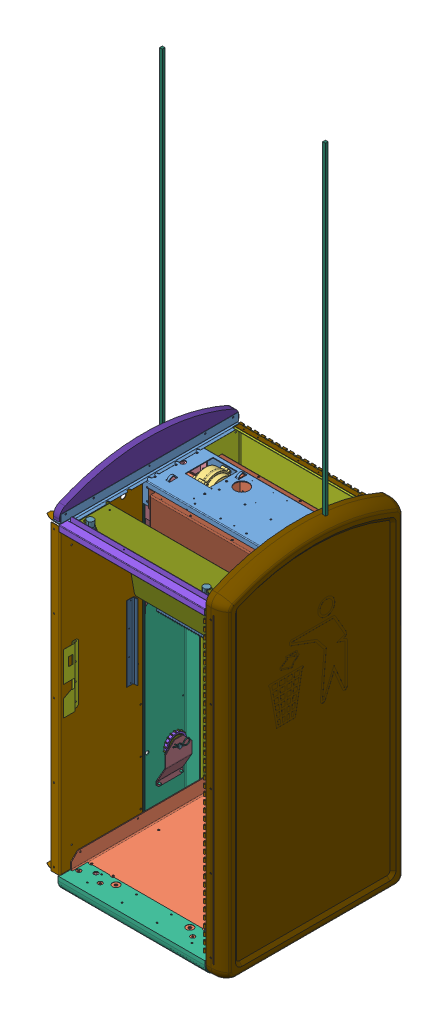
SolidWorks assembly BB3_Assy_Meca_3D, configuration Défaut. Lengths in mm.
Overall size (667 1195.8 661.5).
120 component instances, 56 part files, 9 mates.
Components (placement in the parent):
- BB3_Chassis-1: BB3_Chassis [Défaut] at (-140.0351 388.7943 -82.8142) size (675.82 1282.03 663.93)
  - TopCrossmember_Rev2-1: TopCrossmember_Rev2 [Default] at (20.5473 102.5902 0) size (635 86.99 210.82)
  - TopCrossMotorBrkt_Rev3-1: TopCrossMotorBrkt_Rev3 [Défaut] at (-101.9976 61.051 0) size (152.4 200.54 205.51)
  - Moto_Reducteur_011_562_1_216-1: Moto_Reducteur_011_562_1_216 [Default] at (192.9322 74.2423 -36.8146) x (0 -0.000019 -1) z (-1 0 0) size (114.3 226.4 239.81)
  - TopCrossBearingBrkt_Rev1-1: TopCrossBearingBrkt_Rev1 [Défaut] at (-246.0257 61.051 0) size (25.4 73.66 205.51)
  - TopCrossBearingBrkt_Rev1-2: TopCrossBearingBrkt_Rev1 [Défaut] at (287.1203 61.051 0) x (-1 0 0) z (0 0 -1) size (25.4 73.66 205.51)
  - Chassis_Coussinet-1: Chassis_Coussinet [Default] at (-247.5497 60.2788 -36.8146) x (0 -0.995993 0.089436) z (0 0.089436 0.995993) size (28.27 19.05 28.27)
  - Chassis_Coussinet-2: Chassis_Coussinet [Default] at (288.6443 60.2788 -36.8146) x (0 0.997938 0.064185) z (0 -0.064185 0.997938) size (28.27 19.05 28.27)
  - Chassis_Support_Moteur-1: Chassis_Support_Moteur [Défaut] at (-296.9017 100.6288 0.0002) x (0 0 1) z (0 1 0) size (205.51 54 1127)
  - Chassis_Support_Moteur-2: Chassis_Support_Moteur [Défaut] at (337.9963 100.6288 0.0002) x (0 0 -1) z (0 1 0) size (205.51 54 1127)
  - Chassis_Panneau_Arriere-2: Chassis_Panneau_Arriere [Défaut] at (20.5983 -479.4712 -246.619) x (0 0 1) z (0 1 0) size (164.98 667 1155.29)
  - Chassis_Support_Batterie-2: Chassis_Support_Batterie [Défaut] at (20.5983 -270.8192 -242.544) x (0 0 1) z (-1 0 0) size (116.32 446 529)
  - Chassis_Support_Moteur_Devant_Gauche-2: Chassis_Support_Moteur_Devant_Gauche [Défaut] at (-249.8894 -442.8187 130.7585) x (0 0 -1) z (0 1 0) size (329.85 66 1105)
  - Chassis_Positionnement_Emetteur_Recepteur_Gauche-2: Chassis_Positionnement_Emetteur_Recepteur_Gauche [Défaut] at (-222.4622 -381.8185 156.8606) x (1 0 0) z (0 -1 0) size (22.1 48.5 273)
  - Chassis_Support_Moteur_Devant_Droite-1: Chassis_Support_Moteur_Devant_Droite [Défaut] at (290.9839 -442.8187 130.7585) x (0 0 -1) z (0 -1 0) size (329.85 66 1105)
  - Chassis_Positionnement_Emetteur_Recepteur_Droite-1: Chassis_Positionnement_Emetteur_Recepteur_Droite [Défaut] at (263.5568 -381.8185 156.8606) x (-1 0 0) z (0 1 0) size (22.1 48.5 273)
  - Chassis_Support_Pignon_bas-1: Chassis_Support_Pignon_bas [Défaut] at (305.4963 -865.3715 -39.8528) x (-1 0 0) z (0 0 1) size (35.2 151.29 95)
  - Chassis_Axe_Pignon_Bas-1: Chassis_Axe_Pignon_Bas [Défaut] at (340.9963 -816.3715 -39.8528) x (-1 0 0) z (0 -0.052233 -0.998635) size (48.6 15.9 15.9)
  - Chassis_Goupille_Axe_Pignon_bas-1: Chassis_Goupille_Axe_Pignon_bas [Défaut] at (300.5463 -817.6251 -63.8201) x (0 0.052233 0.998635) z (1 0 0) size (60.5 23 3)
  - Chassis_Support_Pignon_bas-2: Chassis_Support_Pignon_bas [Défaut] at (-264.4017 -865.3715 -39.8528) x (1 0 0) z (0 0 -1) size (35.2 151.29 95)
  - Chassis_Axe_Pignon_Bas-2: Chassis_Axe_Pignon_Bas [Défaut] at (-299.9017 -816.3715 -39.8528) x (1 0 0) z (0 0.31653 0.948583) size (48.6 15.9 15.9)
  - Chassis_Goupille_Axe_Pignon_bas-2: Chassis_Goupille_Axe_Pignon_bas [Défaut] at (-259.4517 -808.7748 -17.0869) x (0 -0.31653 -0.948583) z (1 0 0) size (60.5 23 3)
  - Chassis_Plaque_Haute-1: Chassis_Plaque_Haute [Défaut] at (20.4963 92.768 412.6062) x (0 0 -1) z (1 0 0) size (278.51 354.1 562.7)
  - Chassis_Renfort-1: Chassis_Renfort [Défaut] at (20.5463 -1018.8712 0.0002) x (0 0 1) z (-1 0 0) size (199.51 39 641)
  - Chassis_Charniere_Photovoltaique-1: Chassis_Charniere_Photovoltaique [Défaut] at (20.5983 134.4053 -220.1468) x (0 0 -1) z (1 0 0) size (21.77 6 520)
  - Chassis_Equerre_Haute-1: Chassis_Equerre_Haute [Défaut] at (-246.1446 112.2812 81.6782) x (1 0 0.000001) z (-0.000001 0 1) size (44 37.45 648)
  - Chassis_Equerre_Haute-2: Chassis_Equerre_Haute [Défaut] at (287.2893 112.2812 81.6751) x (-1 0 -0.000168) z (0.000168 0 -1) size (44 37.45 648)
  - Chassis_Repose_Bac_Dechets-1: Chassis_Repose_Bac_Dechets [Défaut] at (20.4963 -992.8728 80.2436) x (0 -0.000001 1) z (-1 0 0) size (641.73 77 529)
  - Chassis_Semelle-1: Chassis_Semelle [Défaut] at (20.4963 -1034.3925 80.4561) x (1 0 0) z (0 -0.000001 1) size (404.15 56 558)
  - Chassis_Repose_Pied-1: Chassis_Repose_Pied [Défaut] at (-187.0037 -1049.3185 336.4561) x (1 0 0) z (0 -0.000001 1) size (94 52.5 63.3)
  - Chassis_Repose_Pied-2: Chassis_Repose_Pied [Défaut] at (-187.0037 -1049.3182 -175.5439) x (1 0 0) z (0 -0.000001 1) size (94 52.5 63.3)
  - Chassis_Repose_Pied-3: Chassis_Repose_Pied [Défaut] at (227.9963 -1049.3182 -175.5439) x (1 0 0) z (0 -0.000001 1) size (94 52.5 63.3)
  - Chassis_Repose_Pied-4: Chassis_Repose_Pied [Défaut] at (227.9963 -1049.3185 336.4561) x (1 0 0) z (0 -0.000001 1) size (94 52.5 63.3)
  - Chassis_Repose_Pied_Insert-1: Chassis_Repose_Pied_Insert [Défaut] at (-187.0037 -1050.3185 336.4561) x (0 1 0.000001) z (0.428959 -0.000001 0.903324) size (14.3 17.5 17.5)
  - Chassis_Repose_Pied_Insert-2: Chassis_Repose_Pied_Insert [Défaut] at (227.9963 -1050.3185 336.4561) x (0 1 0.000001) z (0.384049 -0.000001 0.923313) size (14.3 17.5 17.5)
  - Chassis_Repose_Pied_Insert-3: Chassis_Repose_Pied_Insert [Défaut] at (227.9963 -1050.3182 -175.5439) x (0 1 0.000001) z (-0.000001 -0.000001 1) size (14.3 17.5 17.5)
  - Chassis_Repose_Pied_Insert-4: Chassis_Repose_Pied_Insert [Défaut] at (-187.0037 -1050.3182 -175.5439) x (0 1 0.000001) z (-0.000001 -0.000001 1) size (14.3 17.5 17.5)
  - Chassis_Repose_Pied_Insert-5: Chassis_Repose_Pied_Insert [Défaut] at (-114.0037 -995.8185 336.4561) x (0 -1 -0.000001) z (0.798225 0 0.602359) size (14.3 17.5 17.5)
  - Chassis_Repose_Pied_Insert-6: Chassis_Repose_Pied_Insert [Défaut] at (154.9963 -995.8185 336.4561) x (0 -1 -0.000001) z (0.000001 -0.000001 1) size (14.3 17.5 17.5)
  - Chassis_Repose_Pied_Insert-7: Chassis_Repose_Pied_Insert [Défaut] at (-114.0037 -995.8182 -175.5439) x (0 -1 -0.000001) z (0.000001 -0.000001 1) size (14.3 17.5 17.5)
  - Chassis_Repose_Pied_Insert-8: Chassis_Repose_Pied_Insert [Défaut] at (154.9963 -995.8182 -175.5439) x (0 -1 -0.000001) z (0.000001 -0.000001 1) size (14.3 17.5 17.5)
  - Chassis_Dessous_Avant_Porte-1: Chassis_Dessous_Avant_Porte [Défaut] at (20.4963 -992.8728 80.2436) x (0 -0.000001 1) z (-1 0 0) size (98 53.79 536)
  - Chassis_Serrure-1: Chassis_Serrure [Défaut] at (-243.4017 -382.964 366.4072) x (1 0 0) z (0 1 0) size (10.5 63.82 216)
  - Chassis_Equerre_Face-1: Chassis_Equerre_Face [Défaut] at (20.4963 111.0096 411.9878) x (0 0 1) z (-1 0 0) size (32.2 41.42 529)
  - Chassis_Charniere_Support_Moteur_Devant_Droite-1: Chassis_Charniere_Support_Moteur_Devant_Droite [Défaut] at (260.2718 -465.3185 388.412) x (0 0 1) z (0 -1 0) size (21.77 6 1066)
  - Chassis_Serrure_Cle-1: Chassis_Serrure_Cle [Défaut] at (-191.3537 126.1269 363.7894) x (0 1 0) z (-1 0 0) size (41.58 38.56 38.97)
    - Chassis_Serrure_Came-1: Chassis_Serrure_Came [Défaut] at (-18.246 14.5659 16.3878) x (0 -1 0) z (1 0 0) size (12.45 12.01 13.54)
    - Chassis_Serrure_Rondelle_Ecrou-1: Chassis_Serrure_Rondelle_Ecrou [Défaut] at (-31.074 17.7899 -9.8703) x (0 0.096744 0.995309) z (-1 0 0) size (35.31 35.31 0.64)
    - Chassis_Serrure_Ecrou_Hex-1: Chassis_Serrure_Ecrou_Hex [Défaut] at (-26.3115 -31.157 8.2014) x (0 0 1) z (-1 0 0) size (33 28.58 4.76)
    - Chassis_Serrure_Insert_Cle-1: Chassis_Serrure_Insert_Cle [Défaut] at (26.379 -212.8643 14.6) x (-1 0 0) z (0 0 -1) size (23.33 15.95 15.95)
    - Chassis_Serrure_Support-1: Chassis_Serrure_Support [Défaut] at (-26.6815 11.1833 12.473) x (-1 0 0) z (0 -1 0) size (41.46 28.7 28.7)
    - Chassis_Serrure_Ressort-1: Chassis_Serrure_Ressort [Défaut] at (-1.4058 10.243 9.1044) x (0 0 -1) z (1 0 0) size (21.49 4.59 4.57)
    - Chassis_Serrure_Pene-1: Chassis_Serrure_Pene [Défaut] at (1.0072 5.2825 -10.1896) x (0 -0.999973 -0.007317) z (-1 0 0) size (16.91 23.47 9.63)
  - Chassis_Serrure_Cle-2: Chassis_Serrure_Cle [Défaut] at (232.3463 126.1269 341.4229) x (0 1 0) z (1 0 0) size (41.58 38.56 38.97)
    - Chassis_Serrure_Came-1: Chassis_Serrure_Came [Défaut] at (-18.246 14.5659 16.3878) x (0 -1 0) z (1 0 0) size (12.45 12.01 13.54)
    - Chassis_Serrure_Rondelle_Ecrou-1: Chassis_Serrure_Rondelle_Ecrou [Défaut] at (-31.074 17.7899 -9.8703) x (0 0.096744 0.995309) z (-1 0 0) size (35.31 35.31 0.64)
    - Chassis_Serrure_Ecrou_Hex-1: Chassis_Serrure_Ecrou_Hex [Défaut] at (-26.3115 -31.157 8.2014) x (0 0 1) z (-1 0 0) size (33 28.58 4.76)
    - Chassis_Serrure_Insert_Cle-1: Chassis_Serrure_Insert_Cle [Défaut] at (26.379 -212.8643 14.6) x (-1 0 0) z (0 0 -1) size (23.33 15.95 15.95)
    - Chassis_Serrure_Support-1: Chassis_Serrure_Support [Défaut] at (-26.6815 11.1833 12.473) x (-1 0 0) z (0 -1 0) size (41.46 28.7 28.7)
    - Chassis_Serrure_Ressort-1: Chassis_Serrure_Ressort [Défaut] at (-1.4058 10.243 9.1044) x (0 0 -1) z (1 0 0) size (21.49 4.59 4.57)
    - Chassis_Serrure_Pene-1: Chassis_Serrure_Pene [Défaut] at (1.0072 5.2825 -10.1896) x (0 -0.999973 -0.007317) z (-1 0 0) size (16.91 23.47 9.63)
  - Tombstone_Rev1-1: Tombstone_Rev1 [Default] at (288.5894 129.5652 81.0473) x (1 0 0.000168) z (-0.000168 0 1) size (22.23 105.62 654.05)
  - Tombstone_Rev1-2: Tombstone_Rev1 [Default] at (-247.4446 129.5652 82.3062) x (-1 0 -0.000001) z (0.000001 0 -1) size (22.23 105.62 654.05)
  - SideSkin_Rev1-1: SideSkin_Rev1 [Default] at (-317.3073 -1045.6118 82.3061) x (-1 0 -0.000001) z (0.000001 0 -1) size (69.87 1274.83 660.4) (hidden)
  - SideSkin_Rev1-2: SideSkin_Rev1 [Default] at (358.4521 -1045.6118 81.059) x (1 0 0.000168) z (-0.000168 0 1) size (69.87 1274.83 660.4)
  - Chassis_Interieur_Cache_Chaine-1: Chassis_Interieur_Cache_Chaine [Défaut] at (-242.9017 -763.8184 0) x (0 -0.000001 1) z (-1 0 0) size (249 989 21) (hidden)
  - Chassis_Interieur_Cache_Chaine-2: Chassis_Interieur_Cache_Chaine [Défaut] at (283.9963 -763.8185 0.0002) x (0 0 -1) z (1 0 0) size (249 989 21)
  - Chassis_Bac_Dechets-1: Chassis_Bac_Dechets [Défaut] at (19.5983 -711.9931 65.1059) x (-1 0 0) z (0 0.000001 -1) size (517 387.96 620.45) (hidden)
- BB3_Axe_Moteur-1: BB3_Axe_Moteur [Défaut] at (-118.6236 449.4588 -117.6952) size (601.11 82.55 82.55)
  - TransmissionShaft_Rev1-1: TransmissionShaft_Rev1 [Défaut] at (-0.7672 -0.3857 -1.9336) size (596.9 18.75 19.05)
  - CounterDisc_Rev1-1: CounterDisc_Rev1 [Défaut] at (188.8209 -0.3857 -1.9336) size (0.91 82.55 82.55)
  - Pignon_Haut-1: Pignon_Haut [Défaut] at (-297.0312 -0.3857 -1.9336) x (0 0 1) z (-1 0 0) (suppressed, hidden)
  - Pignon_Haut-2: Pignon_Haut [Défaut] at (294.0828 -0.3857 -1.9336) x (0 0 -1) z (1 0 0) (suppressed, hidden)
  - SHAFT_COLLAR_MCMASTER_6166K28-1: SHAFT_COLLAR_MCMASTER_6166K28 [Défaut] at (181.6772 -0.3857 -1.9336) size (14.29 38.1 38.1)
  - TRANSMISSION_KEY_MC_98870A140-1: TRANSMISSION_KEY_MC_98870A140 [Défaut] at (-285.8172 18.6654 -1.9336) x (-1 0 0) z (0 0 1) size (25.4 4.76 4.76)
  - TRANSMISSION_KEY_MC_98870A140-2: TRANSMISSION_KEY_MC_98870A140 [Défaut] at (284.2828 18.6654 -1.9336) x (-1 0 0) z (0 0 1) size (25.4 4.76 4.76)
  - TRANSMISSION_KEY_MC_98870A190-1: TRANSMISSION_KEY_MC_98870A190 [Défaut] at (-155.0672 18.6654 -1.9336) x (-1 0 0) z (0 0 1) size (63.5 4.76 4.76)
  - PURPLE_IGUS-1: PURPLE_IGUS [Défaut] at (191.2568 -0.3857 -1.9336) x (0 0.381849 -0.924225) z (0 0.924225 0.381849) size (28.27 19.05 28.27)
  - BB3_Pignon_Cylindre_Primitif-1: BB3_Pignon_Cylindre_Primitif [Défaut] at (-295.6312 -0.3857 -1.9336) x (0 0 -1) z (1 0 0) size (73.14 73.14 10)
  - BB3_Pignon_Cylindre_Primitif-2: BB3_Pignon_Cylindre_Primitif [Défaut] at (295.4828 -0.3857 -1.9336) x (0 0 -1) z (1 0 0) size (73.14 73.14 10)
  - Pignon_Haut-3: Pignon_Haut [Défaut] at (-297.0312 -0.3857 -1.9336) x (0 0 1) z (-1 0 0)
  - Pignon_Haut-4: Pignon_Haut [Défaut] at (296.8828 -0.3857 -1.9336) x (0 0 -1) z (1 0 0)
- BB3_Rame_Compacteur-1: BB3_Rame_Compacteur [Défaut] at (-143.8198 251.6092 -80.1568) size (627.3 1739.7 268.31)
  - Compacteur_Rame-1: Compacteur_Rame [Défaut] at (24.383 25.4321 -2.9042) size (505.8 287.44 265.81)
  - Compacteur_Flasque-1: Compacteur_Flasque [Défaut] at (23.883 58.9321 129.5958) x (-1 0 0) z (0 0 -1) size (481.4 343 21.8)
  - Compacteur_Flasque-2: Compacteur_Flasque [Défaut] at (24.883 58.9321 -135.4042) size (481.4 343 21.8)
  - Compacteur_Guide_Droit-1: Compacteur_Guide_Droit [Défaut] at (297.583 154.6611 -2.9042) x (0 0 1) z (0 -1 0) size (185.61 92.3 356)
  - Compacteur_Guide_Gauche-1: Compacteur_Guide_Gauche [Défaut] at (-250.117 154.6611 -2.9042) x (0 0 -1) z (0 -1 0) size (185.61 93.6 356)
  - Compacteur_Guide_Patin-1: Compacteur_Guide_Patin [Défaut] at (-270.917 -23.3389 -95.7102) x (-1 0 0) z (0 0 -1) size (38 350 6.7)
  - Compacteur_Guide_Patin-2: Compacteur_Guide_Patin [Défaut] at (-270.917 -23.3389 89.9018) size (38 350 6.7)
  - Compacteur_Guide_Patin-3: Compacteur_Guide_Patin [Défaut] at (318.383 -23.3389 89.9018) size (38 350 6.7)
  - Compacteur_Guide_Patin-4: Compacteur_Guide_Patin [Défaut] at (318.383 -23.3389 -95.7102) x (-1 0 0) z (0 0 -1) size (38 350 6.7)
  - BB3_Coulissant_Vertical_Cremaillere-1: BB3_Coulissant_Vertical_Cremaillere [Défaut] at (-273.2835 838.3611 2.0958) x (-1 0 0) z (0 -1 0) size (10 10 1400)
  - BB3_Coulissant_Vertical_Cremaillere-2: BB3_Coulissant_Vertical_Cremaillere [Défaut] at (320.7496 838.3611 2.0958) x (1 0 0) z (0 1 0) size (10 10 1400)
- BB3_Pignon_Bas-1: BB3_Pignon_Bas [Défaut] at (-415.6548 -432.9543 -114.7035) x (0 0 -1) z (1 0 0) size (78.63 79.65 18.29)
  - Pignon_Bas-1: Pignon_Bas [Défaut] at (7.9635 5.3771 0) size (78.63 79.65 11.2)
  - Bearing_203KRR5-1: Bearing_203KRR5 [Défaut] at (7.9635 5.3771 0) x (0 0 -1) z (1 0 0) size (12 56.49 56.49)
    - Bearing_203KRR5_BE-1: Bearing_203KRR5_BE [Défaut] x (-1 0 0) z (0 -0.669852 0.742494) size (12 40 40)
    - Bearing_203KRR5_ER-1: Bearing_203KRR5_ER [Défaut] at (0 10.8207 9.7621) x (1 0 0) z (0 0.742494 0.669852) size (6 6 6)
    - Bearing_203KRR5_ER-2: Bearing_203KRR5_ER [Défaut] at (0 14.3789 -2.3734) x (1 0 0) z (0 0.986649 -0.162859) size (6 6 6)
    - Bearing_203KRR5_ER-3: Bearing_203KRR5_ER [Défaut] at (0 7.1095 -12.7217) x (1 0 0) z (0 0.487837 -0.872935) size (6 6 6)
    - Bearing_203KRR5_ER-4: Bearing_203KRR5_ER [Défaut] at (0 -5.5135 -13.4903) x (1 0 0) z (0 -0.378326 -0.925672) size (6 6 6)
    - Bearing_203KRR5_ER-5: Bearing_203KRR5_ER [Défaut] at (0 -13.9848 -4.1004) x (1 0 0) z (0 -0.959602 -0.28136) size (6 6 6)
    - Bearing_203KRR5_ER-6: Bearing_203KRR5_ER [Défaut] at (0 -11.9252 8.3772) x (1 0 0) z (0 -0.818278 0.574822) size (6 6 6)
    - Bearing_203KRR5_ER-7: Bearing_203KRR5_ER [Défaut] at (0 -0.8857 14.5466) x (1 0 0) z (0 -0.060774 0.998152) size (6 6 6)
  - Bearing_203KRR5_BI-1: Bearing_203KRR5_BI [Défaut] at (7.9635 5.3771 0) x (0 0 -1) z (1 0 0) size (18.29 24.43 24.43)
  - BB3_Pignon_Cylindre_Primitif-1: BB3_Pignon_Cylindre_Primitif [Défaut] at (7.9635 5.3771 1.4) size (73.14 73.14 10)
- BB3_Pignon_Bas-2: BB3_Pignon_Bas [Défaut] at (178.2592 -432.9543 -130.6306) x (0 0 1) z (-1 0 0) size (78.63 79.65 18.29)
  - Pignon_Bas-1: Pignon_Bas [Défaut] at (7.9635 5.3771 0) size (78.63 79.65 11.2)
  - Bearing_203KRR5-1: Bearing_203KRR5 [Défaut] at (7.9635 5.3771 0) x (0 0 -1) z (1 0 0) size (12 56.49 56.49)
    - Bearing_203KRR5_BE-1: Bearing_203KRR5_BE [Défaut] x (-1 0 0) z (0 -0.669852 0.742494) size (12 40 40)
    - Bearing_203KRR5_ER-1: Bearing_203KRR5_ER [Défaut] at (0 10.8207 9.7621) x (1 0 0) z (0 0.742494 0.669852) size (6 6 6)
    - Bearing_203KRR5_ER-2: Bearing_203KRR5_ER [Défaut] at (0 14.3789 -2.3734) x (1 0 0) z (0 0.986649 -0.162859) size (6 6 6)
    - Bearing_203KRR5_ER-3: Bearing_203KRR5_ER [Défaut] at (0 7.1095 -12.7217) x (1 0 0) z (0 0.487837 -0.872935) size (6 6 6)
    - Bearing_203KRR5_ER-4: Bearing_203KRR5_ER [Défaut] at (0 -5.5135 -13.4903) x (1 0 0) z (0 -0.378326 -0.925672) size (6 6 6)
    - Bearing_203KRR5_ER-5: Bearing_203KRR5_ER [Défaut] at (0 -13.9848 -4.1004) x (1 0 0) z (0 -0.959602 -0.28136) size (6 6 6)
    - Bearing_203KRR5_ER-6: Bearing_203KRR5_ER [Défaut] at (0 -11.9252 8.3772) x (1 0 0) z (0 -0.818278 0.574822) size (6 6 6)
    - Bearing_203KRR5_ER-7: Bearing_203KRR5_ER [Défaut] at (0 -0.8857 14.5466) x (1 0 0) z (0 -0.060774 0.998152) size (6 6 6)
  - Bearing_203KRR5_BI-1: Bearing_203KRR5_BI [Défaut] at (7.9635 5.3771 0) x (0 0 -1) z (1 0 0) size (18.29 24.43 24.43)
  - BB3_Pignon_Cylindre_Primitif-1: BB3_Pignon_Cylindre_Primitif [Défaut] at (7.9635 5.3771 1.4) size (73.14 73.14 10)
Mates (geometry in assembly coordinates):
- Coaxiale1: concentric anti-aligned: cylinder of BB3_Chassis-1/Chassis_Coussinet-1 through (-387.5848 449.0731 -119.6288) axis (1 0 0) radius 9.6139; cylinder of BB3_Axe_Moteur-1/TransmissionShaft_Rev1-1 through (179.0592 449.0731 -119.6288) axis (-1 0 0) radius 9.525
- Distance1: distance = 9.56 mm anti-aligned: plane of BB3_Axe_Moteur-1/Pignon_Haut-3 through (-397.1448 449.0731 -119.6288) normal (1 0 0); plane of BB3_Chassis-1/Chassis_Coussinet-1 through (-387.5848 449.0731 -119.6288) normal (-1 0 0)
- Coïncidente2: coincident aligned: plane of BB3_Chassis-1/Chassis_Panneau_Arriere-2; plane of BB3_Rame_Compacteur-1/Compacteur_Rame-1 through (-119.4368 277.0413 -83.061) normal (1 0 0)
- Coïncidente3: coincident anti-aligned: plane of BB3_Chassis-1/Chassis_Support_Moteur-1 through (-385.9368 -637.5769 -182.567) normal (0 0 1); plane of BB3_Rame_Compacteur-1/Compacteur_Guide_Patin-1 through (-414.7368 228.2703 -182.567) normal (0 0 -1)
- Distance2: distance = 12 mm aligned: plane of BB3_Rame_Compacteur-1/Compacteur_Flasque-2 through (-335.4368 482.0413 -215.561) normal (0 1 0); plane of BB3_Chassis-1/TopCrossmember_Rev2-1 through (-436.9878 494.0413 22.5958) normal (0 1 0)
- Coaxiale2: concentric anti-aligned: cylinder of BB3_Chassis-1/Chassis_Axe_Pignon_Bas-2 through (-417.6368 -427.5772 -122.667) axis (1 0 0) radius 6.25; cylinder of BB3_Pignon_Bas-1/Bearing_203KRR5_BI-1 through (-415.6548 -427.5772 -122.667) axis (-1 0 0) radius 6.5405
- Coïncidente5: coincident aligned: plane of BB3_Axe_Moteur-1/Pignon_Haut-3 through (-419.2548 469.8587 -119.6288) normal (-1 0 0); plane of BB3_Pignon_Bas-1/Pignon_Bas-1 through (-419.2548 -406.7916 -122.667) normal (-1 0 0)
- Coaxiale3: concentric anti-aligned: cylinder of BB3_Chassis-1/Chassis_Axe_Pignon_Bas-1 through (178.6612 -427.5772 -122.667) axis (-1 0 0) radius 6.25; cylinder of BB3_Pignon_Bas-2/Bearing_203KRR5_BI-1 through (178.2592 -427.5772 -122.667) axis (1 0 0) radius 6.5405
- Coïncidente6: coincident aligned: plane of BB3_Axe_Moteur-1/Pignon_Haut-4 through (181.8592 469.8587 -119.6288) normal (1 0 0); plane of BB3_Pignon_Bas-2/Pignon_Bas-1 through (181.8592 -406.7916 -122.667) normal (1 0 0)
